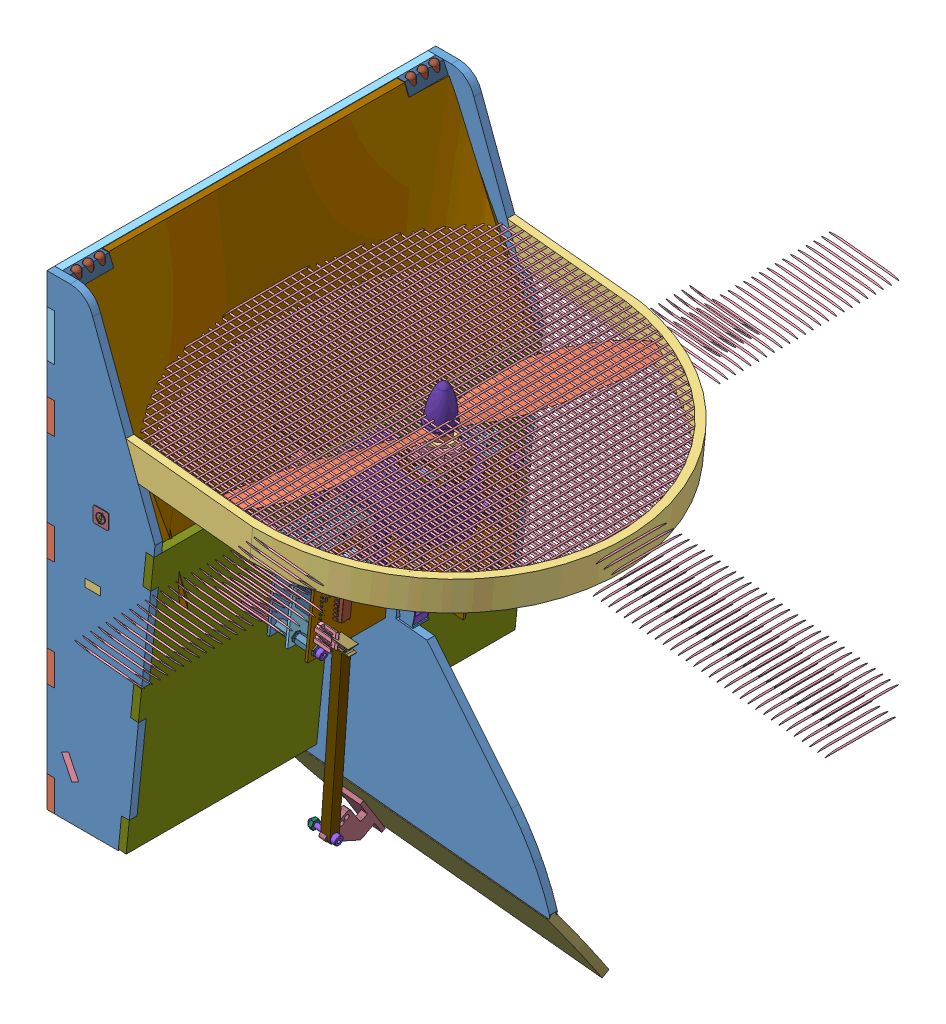
SolidWorks assembly AssTotaleSimu6, configuration Défaut. Lengths in mm. (continued)
Components (placement in the parent): (continued)
- AssStructSimu-1: AssStructSimu [Défaut] at (-125.7658 -1.8483 624.6548) x (1 0 0) z (0 0 -1) size (253.25 324.59 251.6) (continued)
  - AssCarte-1: AssCarte [Défaut] at (38.0121 147.1029 290.772) x (-0.101852 0.9948 0) z (0.9948 0.101852 0) size (66.52 130.57 98.72) (continued)
    - AssEntretoise-3: AssEntretoise [Défaut] at (-106.8199 -51.2976 37.1344) x (0 0 -1) z (1 0 0) size (58.24 7.29 7.81)
      - socket head cap screw 4762_din-1: socket head cap screw 4762_din [EN ISO 4762 M3 x 5 - 5N] at (-2.4967 0.5867 0) size (8 5.5 5.5)
      - hexagonal_spacer_MF_M3_H20_HEX5.5_FTD6_MTL6-1: hexagonal_spacer_MF_M3_H20_HEX5.5_FTD6_MTL6 [Défaut] at (48.3433 0.5867 0) x (0 0 1) z (-1 0 0) size (6.36 5.51 26)
      - hex nut style 1 gradeab_din-1: hex nut style 1 gradeab_din [Hexagon Nut ISO 4032 - M3 - W - N] at (53.3433 0.5867 0) x (0 0.943962 0.330053) z (-1 0 0) size (5.5 6.35 2.4)
      - hexagonal_spacer_MF_M3_H12_HEX5.5_FTD6_MTL6-2: hexagonal_spacer_MF_M3_H12_HEX5.5_FTD6_MTL6 [Défaut] at (27.0633 0.5867 0) x (0 0.248308 0.968681) z (-1 0 0) size (6.36 5.51 18)
      - hexagonal_spacer_MF_M3_H12_HEX5.5_FTD6_MTL6-3: hexagonal_spacer_MF_M3_H12_HEX5.5_FTD6_MTL6 [Défaut] at (13.7833 0.5867 0) x (0 0 1) z (-1 0 0) size (6.36 5.51 18)
    - AssEntretoise-4: AssEntretoise [Défaut] at (-106.8199 68.7024 37.1344) x (0 0 -1) z (1 0 0) size (58.24 7.29 7.81)
      - socket head cap screw 4762_din-1: socket head cap screw 4762_din [EN ISO 4762 M3 x 5 - 5N] at (-2.4967 0.5867 0) size (8 5.5 5.5)
      - hexagonal_spacer_MF_M3_H20_HEX5.5_FTD6_MTL6-1: hexagonal_spacer_MF_M3_H20_HEX5.5_FTD6_MTL6 [Défaut] at (48.3433 0.5867 0) x (0 0 1) z (-1 0 0) size (6.36 5.51 26)
      - hex nut style 1 gradeab_din-1: hex nut style 1 gradeab_din [Hexagon Nut ISO 4032 - M3 - W - N] at (53.3433 0.5867 0) x (0 0.943962 0.330053) z (-1 0 0) size (5.5 6.35 2.4)
      - hexagonal_spacer_MF_M3_H12_HEX5.5_FTD6_MTL6-2: hexagonal_spacer_MF_M3_H12_HEX5.5_FTD6_MTL6 [Défaut] at (27.0633 0.5867 0) x (0 0.248308 0.968681) z (-1 0 0) size (6.36 5.51 18)
      - hexagonal_spacer_MF_M3_H12_HEX5.5_FTD6_MTL6-3: hexagonal_spacer_MF_M3_H12_HEX5.5_FTD6_MTL6 [Défaut] at (13.7833 0.5867 0) x (0 0 1) z (-1 0 0) size (6.36 5.51 18)
    - AssMpu-1: AssMpu [Défaut] at (-150.6881 40.5798 29.6372) x (0.908747 0.417347 0) z (0 0 1) size (8 8 22.28)
      - hex nut style 1 gradeab_din-1: hex nut style 1 gradeab_din [Hexagon Nut ISO 4032 - M3 - W - N] at (0.2783 0.3227 1.2) size (5.5 6.35 2.4)
      - plain washer 6903 type ab_din-1: plain washer 6903 type ab_din [DIN 6903-A3] at (0.2783 0.3227 1.2) x (0 0 1) z (-1 0 0) size (1 8 8)
      - socket head cap screw 4762_din-1: socket head cap screw 4762_din [EN ISO 4762 M3 x 5 - 5N] at (0.2783 0.3227 19.76) x (0 0 -1) z (-0.852155 0.523289 0) size (8 5.5 5.5)
      - hexagonal_spacer_MF_M3_H12_HEX5.5_FTD6_MTL6-1: hexagonal_spacer_MF_M3_H12_HEX5.5_FTD6_MTL6 [Défaut] at (0.2783 0.3227 3.48) size (6.36 5.51 18)
    - AssMpu-2: AssMpu [Défaut] at (-130.3481 40.6665 29.6372) size (8 8 22.28)
      - hex nut style 1 gradeab_din-1: hex nut style 1 gradeab_din [Hexagon Nut ISO 4032 - M3 - W - N] at (0.2783 0.3227 1.2) size (5.5 6.35 2.4)
      - plain washer 6903 type ab_din-1: plain washer 6903 type ab_din [DIN 6903-A3] at (0.2783 0.3227 1.2) x (0 0 1) z (-1 0 0) size (1 8 8)
      - socket head cap screw 4762_din-1: socket head cap screw 4762_din [EN ISO 4762 M3 x 5 - 5N] at (0.2783 0.3227 19.76) x (0 0 -1) z (-0.852155 0.523289 0) size (8 5.5 5.5)
      - hexagonal_spacer_MF_M3_H12_HEX5.5_FTD6_MTL6-1: hexagonal_spacer_MF_M3_H12_HEX5.5_FTD6_MTL6 [Défaut] at (0.2783 0.3227 3.48) size (6.36 5.51 18)
    - AssCosse-1: AssCosse [Défaut] at (-142.6764 26.8797 71.168) x (0 -1 0) z (-0.344896 0 -0.938641) size (9.83 18.66 11.64)
      - socket head cap screw 4762_din-1: socket head cap screw 4762_din [EN ISO 4762 M3 x 6 - 6N] at (-5.1064 0.3659 0) size (9 5.5 5.5)
      - plain washer 6903 type ab_din-1: plain washer 6903 type ab_din [DIN 6903-A3] at (-2.1064 0.3659 0) size (1 8 8)
      - hex nut style 1 gradeab_din-2: hex nut style 1 gradeab_din [Hexagon Nut ISO 4032 - M3 - W - N] at (1.281 0.3659 0) x (0 0.924225 0.381849) z (-1 0 0) size (5.5 6.35 2.4)
      - 31880-1: 31880 [Default] at (0.4936 0.3659 0) x (0 0.344896 -0.938641) z (0 -0.938641 -0.344896) size (5.54 5 17.37)
    - AssCosse-2: AssCosse [Défaut] at (-142.6764 -2.9203 71.168) x (0 -1 0) z (-0.344896 0 -0.938641) size (9.83 18.66 11.64)
      - socket head cap screw 4762_din-1: socket head cap screw 4762_din [EN ISO 4762 M3 x 6 - 6N] at (-5.1064 0.3659 0) size (9 5.5 5.5)
      - plain washer 6903 type ab_din-1: plain washer 6903 type ab_din [DIN 6903-A3] at (-2.1064 0.3659 0) size (1 8 8)
      - hex nut style 1 gradeab_din-2: hex nut style 1 gradeab_din [Hexagon Nut ISO 4032 - M3 - W - N] at (1.281 0.3659 0) x (0 0.924225 0.381849) z (-1 0 0) size (5.5 6.35 2.4)
      - 31880-1: 31880 [Default] at (0.4936 0.3659 0) x (0 0.344896 -0.938641) z (0 -0.938641 -0.344896) size (5.54 5 17.37)
    - AssCosse-3: AssCosse [Défaut] at (-142.6764 12.0797 71.168) x (0 -1 0) z (-0.344896 0 -0.938641) size (9.83 18.66 11.64)
      - socket head cap screw 4762_din-1: socket head cap screw 4762_din [EN ISO 4762 M3 x 6 - 6N] at (-5.1064 0.3659 0) size (9 5.5 5.5)
      - plain washer 6903 type ab_din-1: plain washer 6903 type ab_din [DIN 6903-A3] at (-2.1064 0.3659 0) size (1 8 8)
      - hex nut style 1 gradeab_din-2: hex nut style 1 gradeab_din [Hexagon Nut ISO 4032 - M3 - W - N] at (1.281 0.3659 0) x (0 0.924225 0.381849) z (-1 0 0) size (5.5 6.35 2.4)
      - 31880-1: 31880 [Default] at (0.4936 0.3659 0) x (0 0.344896 -0.938641) z (0 -0.938641 -0.344896) size (5.54 5 17.37)
    - Terminal_QD_Female-1: Terminal_QD_Female [Default] at (-137.2199 31.5422 53.3942) x (0 1 0) z (-1 0 0) size (9.4 5.5 22.35)
    - Terminal_QD_Female-2: Terminal_QD_Female [Default] at (-137.3199 31.5422 36.2942) x (0 -1 0) z (-1 0 0) size (9.4 5.5 22.35)
    - Terminal_QD_Female-3: Terminal_QD_Female [Default] at (-137.2199 1.7422 53.3942) x (0 1 0) z (-1 0 0) size (9.4 5.5 22.35)
    - Terminal_QD_Female-4: Terminal_QD_Female [Default] at (-137.3199 1.7422 35.9942) x (0 1 0) z (-1 0 0) size (9.4 5.5 22.35)
    - Terminal_QD_Female-5: Terminal_QD_Female [Default] at (-137.3199 16.7422 35.9942) x (0 1 0) z (-1 0 0) size (9.4 5.5 22.35)
    - Terminal_QD_Female-6: Terminal_QD_Female [Default] at (-137.2199 16.7422 53.3942) x (0 1 0) z (-1 0 0) size (9.4 5.5 22.35)
- AssTige-1: AssTige [Défaut] at (-241.576 -121.7726 340.4233) x (-0.101791 -0.994204 -0.034587) z (0.9948 -0.101852 0) size (166.39 7.19 19)
  - tige_servo-1: tige_servo [Défaut] at (-106.2712 0.2685 162) size (165 6 6)
  - socket head cap screw 4762_din-2: socket head cap screw 4762_din [EN ISO 4762 M2 x 10 - 10N] at (-104.2712 3.2685 170) x (0 0 -1) z (0.923728 0.383049 0) size (12 3.8 3.8)
  - hex nut style 1 gradeab_din-1: hex nut style 1 gradeab_din [Hexagon Nut ISO 4032 - M3 - W - N] at (55.7288 3.2685 156) size (5.5 6.35 2.4)
  - hex nut style 1 gradeab_din-2: hex nut style 1 gradeab_din [Hexagon Nut ISO 4032 - M2 - W - N] at (-104.2712 3.2685 160) x (0.904801 0.425836 0) z (0 0 1) size (4 4.62 1.6)
  - socket head cap screw 4762_din-3: socket head cap screw 4762_din [EN ISO 4762 M3 x 16 - 16N] at (55.7288 3.2685 171) x (0 0 -1) z (0.923728 0.383049 0) size (19 5.5 5.5)
- AssGoPro-1: AssGoPro [Défaut] at (-119.9926 15.1708 318.2917) x (0 0 -1) z (-0.119031 -0.99289 0) size (64.3 52.3 34.42)
  - GoPRo Frame for LCD Screen-1: GoPRo Frame for LCD Screen [Défaut] at (-2.6935 10.9558 5.5635) size (64.3 47.42 34.42)
    - GoProFrame MJM-1: GoProFrame MJM [Défaut] at (-3.6084 -1.6692 52.45) size (64.3 59.3 23.5)
    - GoPro Hero 3 Front Panel-1: GoPro Hero 3 Front Panel [Défaut] at (-3.6084 -1.6692 55.7) x (-1 0 0) z (0 0 -1) size (59.25 41.2 1.9)
    - GoPro Hero 3 Screen-1: GoPro Hero 3 Screen [Défaut] at (12.7166 3.9308 54.9) size (15 18 1)
    - GoPro Hero 3 Mode Button-1: GoPro Hero 3 Mode Button [Défaut] at (13.4166 -12.4692 54.95) x (-1 0 0) z (0 0 -1) size (11.97 12.11 3.03)
    - GoPro Hero 3 LED Cover-1: GoPro Hero 3 LED Cover [Défaut] at (3.1166 -9.3192 54.85) x (-0.999988 0.004848 0) z (0 0 -1) size (5 5 1.4)
    - GoPro Hero 3 LED Cover-2: GoPro Hero 3 LED Cover [Défaut] at (3.1166 -16.0692 54.85) x (-0.999988 0.004848 0) z (0 0 -1) size (5 5 1.4)
    - GoPro Hero 3 Housing-1: GoPro Hero 3 Housing [Défaut] at (-3.6084 -1.6692 55.7) size (59.37 41.3 29.84)
    - GoPro Hero 3 Lens-1: GoPro Hero 3 Lens [Défaut] at (-18.9334 5.6308 47.35) x (-0.380542 -0.924764 0) z (0 0 -1) size (13.71 15.7 7.94)
    - GoPro Hero 3 Indicator Cover-1: GoPro Hero 3 Indicator Cover [Défaut] at (-25.5834 -22.2692 69.9) x (-0.997412 0 -0.0719) z (0 1 0) size (3 3 2)
    - GoPro Hero 3 Indicator Cover-2: GoPro Hero 3 Indicator Cover [Défaut] at (-28.8834 12.2308 73) x (-0.999992 0.004018 0) z (0 0 1) size (3 3 2)
    - GoPro Hero 3 Indicator Cover-3: GoPro Hero 3 Indicator Cover [Défaut] at (20.6666 16.9308 58.4) x (-0.997739 0 -0.067212) z (0 1 0) size (3 3 2)
    - slot-1: slot [Défaut] at (-24.7434 -9.7363 65.05) x (0 1 0) z (0 0 -1) size (16 15.02 2.44)
    - GoPro Hero 3 HDMI pin-1: GoPro Hero 3 HDMI pin [Défaut] at (-26.982 2.9815 24.7172) x (0.105491 0.98175 -0.158237) z (-0.992872 0.095109 -0.071829) size (3.29 0.86 3.28)
  - support1-2: support1 [Défaut] at (-1.3019 -18.8633 67.0135) x (0 0 1) z (-1 0 0) size (5 5 10)
- AssGouv-1: AssGouv [Défaut] at (-43.2668 -298.2106 479.8345) x (0.9948 -0.101852 0) z (0.055947 0.546439 -0.835628) size (200.18 52.5 43.47)
  - P10_1-1: P10_1 [Défaut] at (-108.1667 -19.4144 197.6829) size (200.18 50.13 5)
  - attache_pale-1: attache_pale [Défaut] at (-49.1667 8.0856 190.1829) x (0 0 -1) z (-1 0 0) size (43.47 35 14)
- Parallax-Servo-Horn-1: Parallax-Servo-Horn [Défaut] at (-69.3162 -29.8353 324.5606) x (0.09792 0.956393 0.27518) z (0.9948 -0.101852 0) size (38.81 38.81 6.17)
- NTM_35-36_engine_assembly-1: NTM_35-36_engine_assembly [Défaut] at (-24.3523 26.8781 325.7101) x (0.9948 -0.101852 0) z (0 0 1) size (60.56 77.2 246.41)
  - engine_base-1: engine_base [Défaut] at (-1.8719 -19.5526 -1.1165) x (0 1 0) z (0 0 1) size (6.8 35 35)
  - engine_bearing-1: engine_bearing [Défaut] at origin size (10 4 10)
  - Propeller_cone-1: Propeller_cone [Défaut] at (-1.8719 33.6474 -4.1165) x (1 0 0) z (0 1 0) size (17.6 17.6 24)
  - engine_bearing-2: engine_bearing [Défaut] at (0 22.8 0) size (10 4 10)
  - NTM_35-36_enginebody-1: NTM_35-36_enginebody [Défaut] at (-1.8719 -12.7526 -1.1165) size (35 31.7 35)
  - Stator-1: Stator [Défaut] at origin size (27.75 22.36 27.94)
  - propellers_10x4-1: propellers_10x4 [Défaut] at (-6.8719 27.4474 -4.9165) size (60.56 10.53 246.41)
  - propeller_washer-1: propeller_washer [Défaut] at (-1.8719 24.4474 -1.1165) x (0 1 0) z (0 0 1) size (2.5 18 18)
  - Propeller_adaptor-1: Propeller_adaptor [Défaut] at (2.1948 17.1101 -3.713) size (23.46 32.5 25)
Mates (geometry in assembly coordinates):
- Coaxiale1: concentric aligned: cylinder of AssStructSimu-1/AssToitMot-1/AssToit-1/P12-1 through (-27.6967 12.5918 324.5936) axis (-0.101852 -0.9948 0) radius 17.5; cylinder of NTM_35-36_engine_assembly-1/NTM_35-36_enginebody-1 through (-25.2217 36.7654 324.5936) axis (-0.101852 -0.9948 0) radius 17.5
- Coïncidente1: coincident anti-aligned: plane of AssStructSimu-1/AssToitMot-1/AssToit-1/P12-1 through (-28.206 7.6178 324.5936) normal (0.101852 0.9948 0); plane of NTM_35-36_engine_assembly-1/engine_bearing-1 through (-28.206 7.6178 324.5936) normal (-0.101852 -0.9948 0)
- Coaxiale2: concentric aligned: cylinder of AssStructSimu-1/AssToitMot-1/AssToit-1/P10_2-1 through (49.7135 -178.7878 324.5936) axis (-0.9948 0.101852 0) radius 2.5; cylinder of AssGouv-1/P10_1-1 through (-94.0351 -164.0702 324.5936) axis (-0.9948 0.101852 0) radius 2.5
- Coïncidente2: coincident aligned: plane of AssStructSimu-1/AssToitMot-1/AssToit-1/P10_2-1 through (-137.5516 -157.1017 322.0936) normal (-0.9948 0.101852 0); plane of AssGouv-1/P10_1-1 through (-137.8791 -160.3008 321.1312) normal (-0.9948 0.101852 0)
- Coaxiale3: concentric aligned: cylinder of AssTige-1/socket head cap screw 4762_din-3 through (-45.5416 -197.7164 335.2292) axis (0.9948 -0.101852 0) radius 1.5; cylinder of AssGouv-1/attache_pale-1 through (-85.9983 -193.5742 335.2292) axis (0.9948 -0.101852 0) radius 1.5
- Coaxiale4: concentric aligned: cylinder of AssStructSimu-1/AssToitMot-1/Parallax-Servo_DUMMY-1 through (-70.6554 -29.6982 324.5606) axis (-0.9948 0.101852 0) radius 2.9845; cylinder of Parallax-Servo-Horn-1 through (-70.6554 -29.6982 324.5606) axis (-0.9948 0.101852 0) radius 2.9845
- Coïncidente3: coincident anti-aligned: plane of AssStructSimu-1/AssToitMot-1/Parallax-Servo_DUMMY-1 through (-74.8246 -29.2713 324.5606) normal (0.9948 -0.101852 0); plane of Parallax-Servo-Horn-1 through (-74.8246 -29.2713 324.5606) normal (-0.9948 0.101852 0)
- Coaxiale5: concentric anti-aligned: cylinder of AssTige-1/socket head cap screw 4762_din-2 through (-30.2498 -38.5418 340.7631) axis (0.9948 -0.101852 0) radius 1; cylinder of Parallax-Servo-Horn-1 through (-69.7931 -34.4932 340.7631) axis (-0.9948 0.101852 0) radius 0.635
- Coïncidente4: coincident anti-aligned: plane of AssTige-1/tige_servo-1 through (-69.6001 -32.608 343.8305) normal (-0.9948 0.101852 0); plane of Parallax-Servo-Horn-1 through (-68.8748 -25.5237 332.3708) normal (0.9948 -0.101852 0)
- Coaxiale6: concentric aligned: cylinder of AssStructSimu-1/AssBase-1/socket head cap screw 4762_din-7 through (-144.5139 -51.9008 369.3436) axis (0 0 1) radius 1.5; cylinder of AssGoPro-1/support1-2 through (-144.5139 -51.9008 319.5936) axis (0 0 1) radius 1.5
- Coïncidente5: coincident anti-aligned: plane of AssStructSimu-1/AssBase-1/support2-1 through (-141.9706 -54.3568 329.5936) normal (0 0 -1); plane of AssGoPro-1/support1-2 through (-146.6985 -49.121 329.5936) normal (0 0 1)
